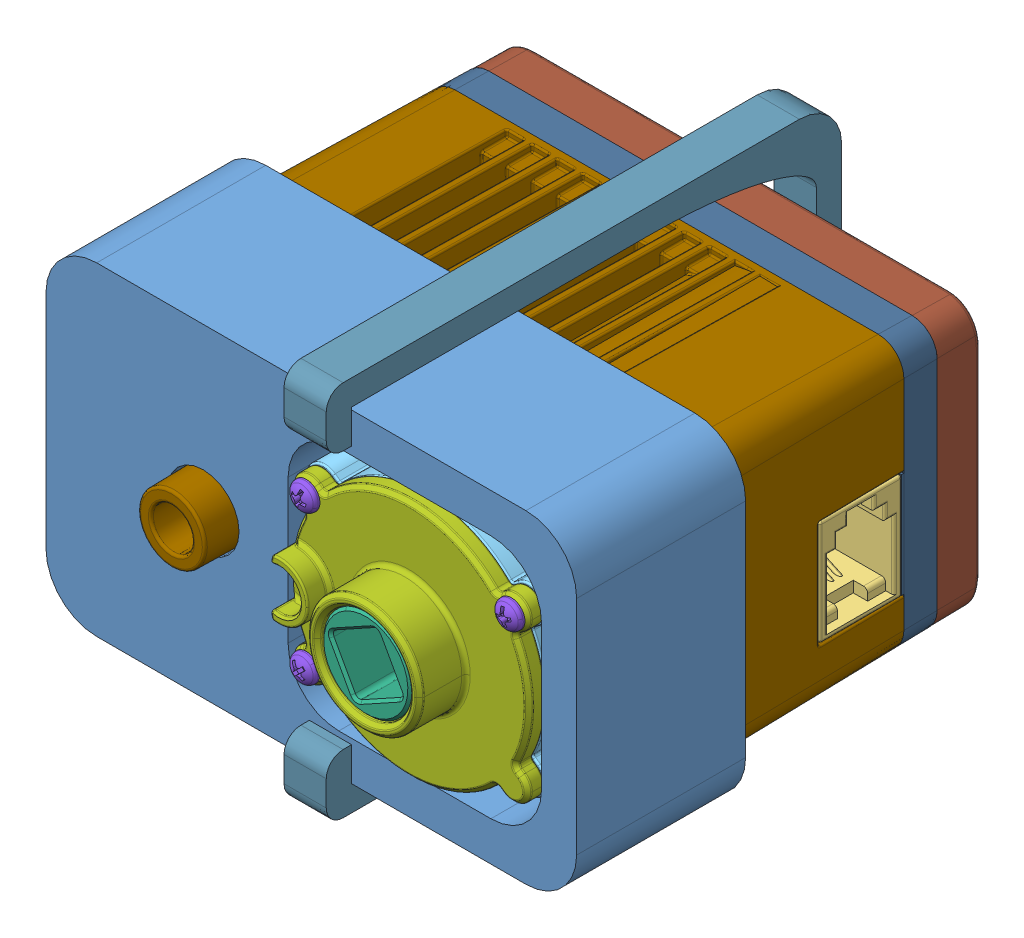
SolidWorks assembly Assem1TestFit, configuration Default. Lengths in mm.
Overall size (62.8 44.6 64.3).
23 component instances, 14 part files, 5 mates.
Components (placement in the parent):
- TestMotorBracket-1: TestMotorBracket [Default] at (-8.633 51.0177 50.7555) size (62.8 38.3 20)
- V5 Smart Motor (276-4840) no cap 3-1: V5 Smart Motor (276-4840) no cap 3 [Default] at (20.017 34.0177 34.5555) size (59.01 35.33 59.91)
  - V5 Smart Motor (276-4840).step-1: V5 Smart Motor (276-4840).step [Default] at origin size (59.01 35.33 59.91)
    - 276-4840-900 Rev6_Instruction.step-1: 276-4840-900 Rev6_Instruction.step [Default] at (-14.3 0 -17.2) size (52.79 15.94 38.15)
      - 276-4840-901 Rev6.step-1: 276-4840-901 Rev6.step [Default] at (10.75 -10.05 17.8) x (-1 0 0) z (0 0 1) size (49.9 1.6 38.15)
      - 276-4840-902 Rev2.step-1: 276-4840-902 Rev2.step [Default] at (31.25 -9.25 6.2) x (0 0 -1) z (0 -1 0) size (10.35 11.39 15.94)
      - 276-4840-022 Rev4.step-1: 276-4840-022 Rev4.step [Default] at (31.25 -9.25 6.2) x (0 0 -1) z (1 0 0) size (10.26 9.1 5.51)
    - 276-4840-110 Rev10_Instruction.step-1: 276-4840-110 Rev10_Instruction.step [Default] at (12.7 0 14.7) size (35.33 35.33 31.1)
      - 276-4840-061 Rev7_Ring_Gear_Fixed01 .6 Rev3.step-1: 276-4840-061 Rev7_Ring_Gear_Fixed01 .6 Rev3.step [Default] at origin size (28.79 28.39 24.6)
      - 276-4840-018 Rev6.step-1: 276-4840-018 Rev6.step [Default] at (0 0 6.7) x (-0.483174 0.875524 0) z (0 0 1) size (26 26 12.3)
      - 276-4840-059 Rev2.step-1: 276-4840-059 Rev2.step [Default] at (0 0 10.3) size (28.4 28.4 8.5)
      - 276-4840-062 Rev1.step-1: 276-4840-062 Rev1.step [Default] at (-12.1353 8.8168 12.3) x (0.956835 -0.290632 0) z (-0.290632 -0.956835 0) size (3.2 6.56 3.2)
      - 276-4840-062 Rev1.step-2: 276-4840-062 Rev1.step [Default] at (12.1353 8.8168 12.3) x (0.978427 0.206591 0) z (0.206591 -0.978427 0) size (3.2 6.56 3.2)
      - 276-4840-062 Rev1.step-3: 276-4840-062 Rev1.step [Default] at (-12.1353 -8.8168 12.3) x (0.72563 0.688086 0) z (0.688086 -0.72563 0) size (3.2 6.56 3.2)
    - 276-4840-001 Rev38.step-1: 276-4840-001 Rev38.step [Default] at origin size (57.3 33 46.9)
    - 276-4840-005 Rev27.step-1: 276-4840-005 Rev27.step [Default] at (0 0 -17.95) size (56.17 31.87 12.9)
    - 276-4840-004 Rev16.step-1: 276-4840-004 Rev16.step [Default] at (0 0 -19.2) size (56.01 31.71 9.21)
    - 276-4840-009 Rev3.step-1: 276-4840-009 Rev3.step [Default] at (25.45 13.5 15.7) x (0.19987 -0.979823 0) z (-0.979823 -0.19987 0) size (3.4 41.31 4.34)
    - 276-4840-009 Rev3.step-2: 276-4840-009 Rev3.step [Default] at (-25.45 -13.5 15.7) x (-0.998855 0.047836 0) z (0.047836 0.998855 0) size (3.4 41.31 4.34)
    - 276-4840-009 Rev3.step-3: 276-4840-009 Rev3.step [Default] at (25.45 -13.5 15.7) x (-0.975374 0.220559 0) z (0.220559 0.975374 0) size (3.4 41.31 4.34)
    - 276-4840-009 Rev3.step-4: 276-4840-009 Rev3.step [Default] at (-25.45 13.5 15.7) x (-0.922256 0.38658 0) z (0.38658 0.922256 0) size (3.4 41.31 4.34)
    - 276-4840-025 Rev19.step-1: 276-4840-025 Rev19.step [Default] at (12.7 0 -22.63) x (-0.993315 0.115437 0) z (0 0 1) size (14.82 14.83 35.18)
- motorRetainerClip-1: motorRetainerClip [Default] at (20.1339 53.7177 60.7555) x (0 0 -1) z (0 -1 0) size (61 5.12 44.6)
Mates (geometry in assembly coordinates):
- Coincident15: coincident aligned: line of TestMotorBracket-1 through (-8.633 47.4177 50.7555) axis (0 -1 0); line of V5 Smart Motor (276-4840) no cap 3-1/V5 Smart Motor (276-4840).step-1/276-4840-001 Rev38.step-1 through (-8.633 46.9177 50.7555) axis (0 -1 0)
- Coincident16: coincident aligned: line of TestMotorBracket-1 through (-5.033 17.5177 50.7555) axis (1 0 0); line of V5 Smart Motor (276-4840) no cap 3-1/V5 Smart Motor (276-4840).step-1/276-4840-001 Rev38.step-1 through (-5.033 17.5177 50.7555) axis (1 0 0)
- Coincident17: coincident anti-aligned: plane of TestMotorBracket-1 through (-8.633 15.1177 60.7555) normal (0 -1 0); plane of motorRetainerClip-1 through (25.1339 15.1177 5.7555) normal (0 1 0)
- Parallel1: parallel anti-aligned: plane of TestMotorBracket-1 through (-8.633 51.0177 60.7555) normal (0 0 1); plane of motorRetainerClip-1 through (25.1339 12.1177 2.7555) normal (0 0 -1)
- Coincident19: coincident anti-aligned: plane of TestMotorBracket-1 through (-8.633 51.0177 60.7555) normal (0 0 1); plane of motorRetainerClip-1 through (25.1339 49.7177 60.7555) normal (0 0 -1)
